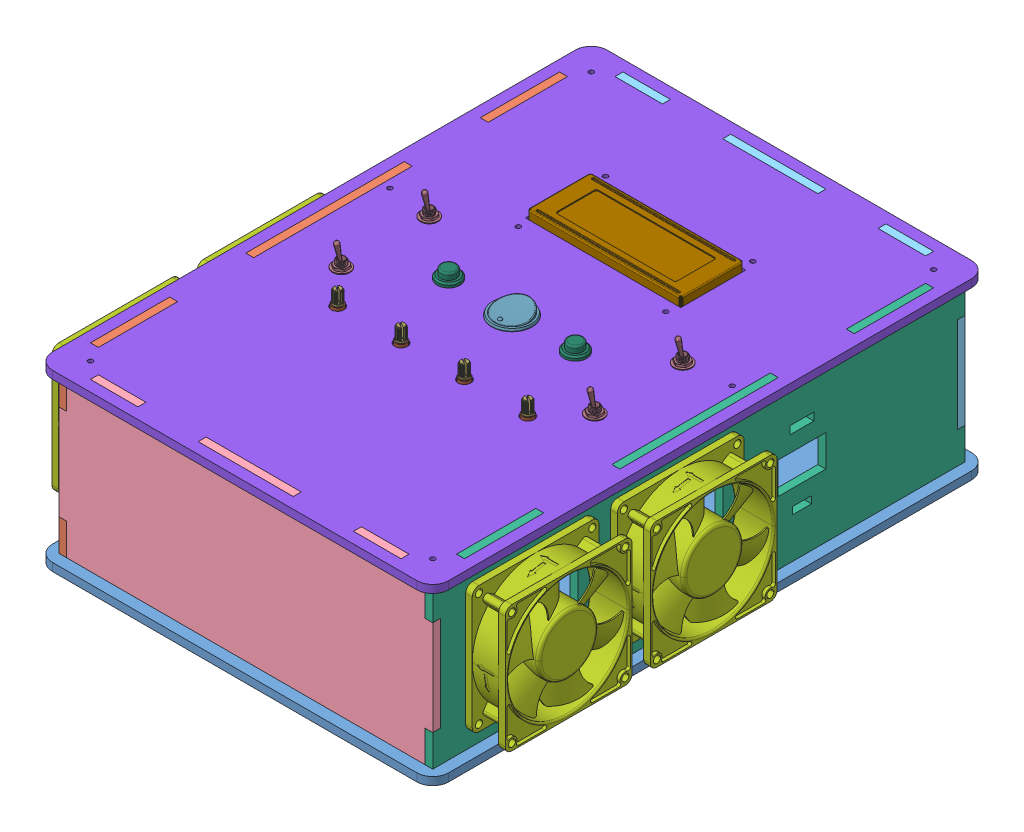
SolidWorks assembly Assem2, configuration Default. Lengths in mm.
Overall size (286.01 126.03 350).
54 component instances, 15 part files, 74 mates.
Components (placement in the parent):
- Bottom2-1: Bottom2 [Default] at (-2.3882 167.7912 456.2901) size (250 5 350)
- LargeEdge-1: LargeEdge [Default] at (9.6118 222.7912 281.2901) x (0 0 1) z (-1 0 0) size (336 110 5)
- PCB_Standoff-1: PCB_Standoff [Default] at (202.4618 172.7912 346.2901) size (4.59 40 5.3)
- PCB_Standoff-2: PCB_Standoff [Default] at (132.6118 172.7912 346.2901) size (4.59 40 5.3)
- PCB_Standoff-3: PCB_Standoff [Default] at (42.7618 172.7912 346.2901) size (4.59 40 5.3)
- PCB_Standoff-4: PCB_Standoff [Default] at (112.6118 172.7912 346.2901) size (4.59 40 5.3)
- PCB_Standoff-5: PCB_Standoff [Default] at (202.4618 172.7912 276.3101) size (4.59 40 5.3)
- PCB_Standoff-6: PCB_Standoff [Default] at (132.6118 172.7912 276.3101) size (4.59 40 5.3)
- PCB_Standoff-7: PCB_Standoff [Default] at (112.6118 172.7912 276.3101) size (4.59 40 5.3)
- PCB_Standoff-8: PCB_Standoff [Default] at (66.7318 172.7912 146.2901) size (4.59 40 5.3)
- PCB_Standoff-9: PCB_Standoff [Default] at (66.7318 172.7912 242.8101) size (4.59 40 5.3)
- PCB_Standoff-10: PCB_Standoff [Default] at (178.4918 172.7912 242.8101) size (4.59 40 5.3)
- PCB_Standoff-11: PCB_Standoff [Default] at (178.4918 172.7912 146.2901) size (4.59 40 5.3)
- PCB_Standoff-12: PCB_Standoff [Default] at (42.7618 172.7912 276.3101) size (4.59 40 5.3)
- SmallEdge-1: SmallEdge [Default] at (122.6118 222.7912 449.2901) x (0 0 -1) z (1 0 0) size (5 110 236)
- SmallEdge_OUTPUT-1: SmallEdge_OUTPUT [Default] at (122.6118 222.7912 118.2901) x (0 0 -1) z (1 0 0) size (5 110 236)
- LargeEdge_Right-1: LargeEdge_Right [Default] at (240.6118 222.7912 281.2901) x (0 0 1) z (-1 0 0) size (336 110 5)
- KARE AKS0YEL FAN_80x80x25 FAN.step-3: KARE AKS0YEL FAN_80x80x25 FAN.step [Default] at (253.1118 222.7912 388.5401) x (0 0 1) z (-1 0 0) size (80.72 80 25.01)
- KARE AKS0YEL FAN_80x80x25 FAN.step-4: KARE AKS0YEL FAN_80x80x25 FAN.step [Default] at (253.1118 222.7912 297.0401) x (0 0 1) z (-1 0 0) size (80.72 80 25.01)
- Top-1: Top [Default] at (-2.3882 272.7912 456.2901) size (250 5 350)
- LCD Display 2004.stp-1: LCD Display 2004.stp [Default] at (122.5938 271.1783 203.0951) size (98.07 13.66 59.94)
- PCB_Standoff_50mm-1: PCB_Standoff_50mm [Default] at (14.6118 172.7912 123.2901) x (0.790641 0 0.61228) z (-0.61228 0 0.790641) size (5.3 50 5.17)
- PCB_Standoff_50mm-2: PCB_Standoff_50mm [Default] at (14.6118 222.7912 123.2901) x (0.790641 0 0.61228) z (-0.61228 0 0.790641) size (5.3 50 5.17)
- PCB_Standoff_50mm-3: PCB_Standoff_50mm [Default] at (230.6118 222.7912 123.2901) size (5.3 50 5.17)
- PCB_Standoff_50mm-4: PCB_Standoff_50mm [Default] at (14.6118 222.7912 250.2901) size (5.3 50 5.17)
- PCB_Standoff_50mm-5: PCB_Standoff_50mm [Default] at (230.6118 172.7912 439.2901) size (5.3 50 5.17)
- PCB_Standoff_50mm-6: PCB_Standoff_50mm [Default] at (230.6118 222.7912 250.2901) size (5.3 50 5.17)
- PCB_Standoff_50mm-7: PCB_Standoff_50mm [Default] at (230.6118 172.7912 250.2901) size (5.3 50 5.17)
- PCB_Standoff_50mm-8: PCB_Standoff_50mm [Default] at (14.6118 172.7912 439.2901) size (5.3 50 5.17)
- PCB_Standoff_50mm-9: PCB_Standoff_50mm [Default] at (14.6118 172.7912 250.2901) size (5.3 50 5.17)
- PCB_Standoff_50mm-10: PCB_Standoff_50mm [Default] at (230.6118 172.7912 123.2901) size (5.3 50 5.17)
- PCB_Standoff_50mm-11: PCB_Standoff_50mm [Default] at (230.6118 222.7912 439.2901) size (5.3 50 5.17)
- PCB_Standoff_50mm-12: PCB_Standoff_50mm [Default] at (14.6118 222.7912 439.2901) size (5.3 50 5.17)
- KARE AKS0YEL FAN_80x80x25 FAN.step-5: KARE AKS0YEL FAN_80x80x25 FAN.step [Default] at (-7.8882 222.7912 297.0401) x (0 0 1) z (-1 0 0) size (80.72 80 25.01)
- KARE AKS0YEL FAN_80x80x25 FAN.step-6: KARE AKS0YEL FAN_80x80x25 FAN.step [Default] at (-7.8882 222.7912 388.5401) x (0 0 1) z (-1 0 0) size (80.72 80 25.01)
- WH148 PH1 Single-Joint Potentiometer.step-1: WH148 PH1 Single-Joint Potentiometer.step [Default] at (62.6118 270.7912 331.2901) x (0.999555 0 0.029816) z (0 1 0) size (16.9 26.15 23.9)
  - Base.step-1: Base.step [Default] at origin size (16.9 26.15 15.6)
  - Knob.step-1: Knob.step [Default] x (0.866025 0.5 0) z (0 0 1) size (5.8 5.8 8.2)
- WH148 PH1 Single-Joint Potentiometer.step-2: WH148 PH1 Single-Joint Potentiometer.step [Default] at (102.6118 270.7912 331.2901) x (1 0 0) z (0 1 0) size (16.9 26.15 23.9)
  - Base.step-1: Base.step [Default] at origin size (16.9 26.15 15.6)
  - Knob.step-1: Knob.step [Default] x (0.866025 0.5 0) z (0 0 1) size (5.8 5.8 8.2)
- WH148 PH1 Single-Joint Potentiometer.step-3: WH148 PH1 Single-Joint Potentiometer.step [Default] at (142.6118 270.7912 331.2901) x (1 0 0) z (0 1 0) size (16.9 26.15 23.9)
  - Base.step-1: Base.step [Default] at origin size (16.9 26.15 15.6)
  - Knob.step-1: Knob.step [Default] x (0.866025 0.5 0) z (0 0 1) size (5.8 5.8 8.2)
- WH148 PH1 Single-Joint Potentiometer.step-4: WH148 PH1 Single-Joint Potentiometer.step [Default] at (182.6118 270.7912 331.2901) x (1 0 0) z (0 1 0) size (16.9 26.15 23.9)
  - Base.step-1: Base.step [Default] at origin size (16.9 26.15 15.6)
  - Knob.step-1: Knob.step [Default] x (0.866025 0.5 0) z (0 0 1) size (5.8 5.8 8.2)
- MTS-102.step-6: MTS-102.step [Default] at (42.6118 273.7912 253.5562) x (0 0 -1) z (1 0 0) size (13.2 33.53 12)
- MTS-102.step-7: MTS-102.step [Default] at (42.6118 273.7912 309.024) x (0 0 -1) z (1 0 0) size (13.2 33.53 12)
- MTS-102.step-8: MTS-102.step [Default] at (202.6118 273.7912 253.5562) x (0 0 -1) z (1 0 0) size (13.2 33.53 12)
- MTS-102.step-9: MTS-102.step [Default] at (202.6118 273.7912 309.024) x (0 0 -1) z (1 0 0) size (13.2 33.53 12)
- rocker switch.step-4: rocker switch.step [Default] at (122.6118 277.7912 281.2901) x (0.999998 0 -0.002169) z (-0.002169 0 -0.999998) size (25.4 25.47 25.4)
- Push Button.step-3: Push Button.step [Default] at (82.6118 268.6912 281.2901) x (1 0 0) z (0 1 0) size (16.28 16.39 30.3)
- Push Button.step-4: Push Button.step [Default] at (162.6118 268.6912 281.2901) x (1 0 0) z (0 1 0) size (16.28 16.39 30.3)
Mates (geometry in assembly coordinates):
- Coincident10: coincident anti-aligned: circle of Bottom2-1; circle of PCB_Standoff-1
- Coincident11: coincident anti-aligned: circle of Bottom2-1; circle of PCB_Standoff-2
- Coincident12: coincident aligned: circle of Bottom2-1; circle of PCB_Standoff-3
- Coincident13: coincident aligned: circle of Bottom2-1; circle of PCB_Standoff-4
- Coincident14: coincident anti-aligned: circle of Bottom2-1; circle of PCB_Standoff-5
- Coincident15: coincident anti-aligned: circle of Bottom2-1; circle of PCB_Standoff-6
- Coincident16: coincident aligned: circle of Bottom2-1; circle of PCB_Standoff-12
- Coincident18: coincident aligned: circle of Bottom2-1; circle of PCB_Standoff-10
- Coincident19: coincident aligned: circle of Bottom2-1; circle of PCB_Standoff-9
- Coincident20: coincident aligned: circle of Bottom2-1; circle of PCB_Standoff-11
- Coincident21: coincident aligned: circle of Bottom2-1; circle of PCB_Standoff-8
- Coincident25: coincident aligned: circle of Bottom2-1; circle of PCB_Standoff-7
- Coincident28: coincident anti-aligned: plane of Bottom2-1 through (220.6118 172.7912 456.2901) normal (-1 0 0); plane of SmallEdge_OUTPUT-1 through (220.6118 222.7912 113.2901) normal (1 0 0)
- Coincident29: coincident anti-aligned: plane of Bottom2-1 through (-2.3882 172.7912 456.2901) normal (0 1 0); plane of SmallEdge_OUTPUT-1 through (122.6118 172.7912 113.2901) normal (0 -1 0)
- Coincident30: coincident anti-aligned: plane of Bottom2-1 through (-2.3882 172.7912 118.2901) normal (0 0 -1); plane of SmallEdge_OUTPUT-1 through (122.6118 222.7912 118.2901) normal (0 0 1)
- Coincident31: coincident anti-aligned: plane of Bottom2-1 through (-2.3882 172.7912 379.2901) normal (0 0 1); plane of LargeEdge-1 through (4.6118 222.7912 379.2901) normal (0 0 -1)
- Coincident32: coincident anti-aligned: plane of Bottom2-1 through (9.6118 172.7912 456.2901) normal (-1 0 0); plane of LargeEdge-1 through (9.6118 222.7912 281.2901) normal (1 0 0)
- Coincident33: coincident anti-aligned: plane of Bottom2-1 through (-2.3882 172.7912 456.2901) normal (0 1 0); plane of LargeEdge-1 through (4.6118 172.7912 281.2901) normal (0 -1 0)
- Coincident34: coincident anti-aligned: plane of Bottom2-1 through (24.6118 172.7912 456.2901) normal (1 0 0); plane of SmallEdge-1 through (24.6118 172.7912 444.2901) normal (-1 0 0)
- Coincident35: coincident anti-aligned: plane of Bottom2-1 through (-2.3882 172.7912 444.2901) normal (0 0 1); plane of SmallEdge-1 through (122.6118 222.7912 444.2901) normal (0 0 -1)
- Coincident36: coincident anti-aligned: plane of Bottom2-1 through (-2.3882 172.7912 456.2901) normal (0 1 0); plane of SmallEdge-1 through (122.6118 172.7912 444.2901) normal (0 -1 0)
- Coincident37: coincident anti-aligned: plane of Bottom2-1 through (-2.3882 172.7912 429.2901) normal (0 0 -1); plane of LargeEdge_Right-1 through (235.6118 222.7912 429.2901) normal (0 0 1)
- Coincident38: coincident anti-aligned: plane of Bottom2-1 through (235.6118 172.7912 456.2901) normal (1 0 0); plane of LargeEdge_Right-1 through (235.6118 222.7912 281.2901) normal (-1 0 0)
- Coincident39: coincident anti-aligned: plane of Bottom2-1 through (-2.3882 172.7912 456.2901) normal (0 1 0); plane of LargeEdge_Right-1 through (235.6118 172.7912 281.2901) normal (0 -1 0)
- Concentric11: concentric aligned: circle of LargeEdge_Right-1; circle of KARE AKS0YEL FAN_80x80x25 FAN.step-3
- Concentric12: concentric aligned: circle of LargeEdge_Right-1; circle of KARE AKS0YEL FAN_80x80x25 FAN.step-3
- Coincident42: coincident anti-aligned: plane of LargeEdge_Right-1 through (240.6118 222.7912 281.2901) normal (1 0 0); plane of KARE AKS0YEL FAN_80x80x25 FAN.step-3 through (240.6118 222.7912 388.5401) normal (-1 0 0)
- Concentric13: concentric aligned: circle of LargeEdge_Right-1; circle of KARE AKS0YEL FAN_80x80x25 FAN.step-4
- Concentric14: concentric aligned: circle of LargeEdge_Right-1; circle of KARE AKS0YEL FAN_80x80x25 FAN.step-4
- Coincident43: coincident anti-aligned: plane of LargeEdge_Right-1 through (240.6118 222.7912 281.2901) normal (1 0 0); plane of KARE AKS0YEL FAN_80x80x25 FAN.step-4 through (240.6118 222.7912 297.0401) normal (-1 0 0)
- Coincident59: coincident anti-aligned: plane of LargeEdge_Right-1 through (235.6118 272.7912 281.2901) normal (0 1 0); plane of Top-1 through (-2.3882 272.7912 447.8511) normal (0 -1 0)
- Concentric25: concentric anti-aligned: cylinder of Top-1 through (76.1118 277.7912 167.3511) axis (0 -1 0) radius 1.5; cylinder of LCD Display 2004.stp-1 through (76.1118 271.1783 167.3511) axis (0 1 0) radius 1.6764
- Parallel7: parallel anti-aligned: plane of Top-1 through (171.6118 277.7912 447.8511) normal (-1 0 0); plane of LCD Display 2004.stp-1 through (170.9681 281.7828 213.3886) normal (1 0 0)
- Coincident61: coincident anti-aligned: plane of Top-1 through (-2.3882 272.7912 447.8511) normal (0 -1 0); plane of LCD Display 2004.stp-1 through (122.5938 272.7912 194.6561) normal (0 1 0)
- Coincident64: coincident aligned: circle of Bottom2-1; circle of PCB_Standoff_50mm-1
- Coincident65: coincident aligned: circle of PCB_Standoff_50mm-1; circle of PCB_Standoff_50mm-2
- Coincident66: coincident aligned: circle of Bottom2-1; circle of PCB_Standoff_50mm-9
- Coincident67: coincident aligned: circle of PCB_Standoff_50mm-4; circle of PCB_Standoff_50mm-9
- Coincident68: coincident anti-aligned: circle of Bottom2-1; circle of PCB_Standoff_50mm-8
- Coincident69: coincident aligned: circle of Bottom2-1; circle of PCB_Standoff_50mm-5
- Coincident70: coincident anti-aligned: circle of Bottom2-1; circle of PCB_Standoff_50mm-7
- Coincident71: coincident anti-aligned: circle of Bottom2-1; circle of PCB_Standoff_50mm-10
- Coincident72: coincident aligned: circle of PCB_Standoff_50mm-3; circle of PCB_Standoff_50mm-10
- Coincident73: coincident aligned: circle of PCB_Standoff_50mm-6; circle of PCB_Standoff_50mm-7
- Coincident74: coincident aligned: circle of PCB_Standoff_50mm-5; circle of PCB_Standoff_50mm-11
- Coincident75: coincident aligned: circle of PCB_Standoff_50mm-8; circle of PCB_Standoff_50mm-12
- Concentric26: concentric anti-aligned: circle of LargeEdge-1; circle of KARE AKS0YEL FAN_80x80x25 FAN.step-5
- Concentric28: concentric anti-aligned: circle of LargeEdge-1; circle of KARE AKS0YEL FAN_80x80x25 FAN.step-5
- Coincident80: coincident anti-aligned: plane of LargeEdge-1 through (4.6118 222.7912 281.2901) normal (-1 0 0); plane of KARE AKS0YEL FAN_80x80x25 FAN.step-5 through (4.6118 222.7912 297.0401) normal (1 0 0)
- Concentric29: concentric anti-aligned: circle of LargeEdge-1; circle of KARE AKS0YEL FAN_80x80x25 FAN.step-6
- Concentric30: concentric anti-aligned: circle of LargeEdge-1; circle of KARE AKS0YEL FAN_80x80x25 FAN.step-6
- Coincident81: coincident anti-aligned: plane of LargeEdge-1 through (4.6118 222.7912 281.2901) normal (-1 0 0); plane of KARE AKS0YEL FAN_80x80x25 FAN.step-6 through (4.6118 222.7912 388.5401) normal (1 0 0)
- Concentric32: concentric anti-aligned: circle of Top-1; circle of WH148 PH1 Single-Joint Potentiometer.step-1/Base.step-1
- Concentric33: concentric anti-aligned: circle of Top-1; circle of WH148 PH1 Single-Joint Potentiometer.step-2/Base.step-1
- Coincident82: coincident anti-aligned: plane of Top-1 through (-2.3882 272.7912 447.8511) normal (0 -1 0); plane of WH148 PH1 Single-Joint Potentiometer.step-2/Base.step-1 through (102.6118 272.7912 322.8511) normal (0 1 0)
- Coincident83: coincident anti-aligned: plane of Top-1 through (-2.3882 272.7912 447.8511) normal (0 -1 0); plane of WH148 PH1 Single-Joint Potentiometer.step-1/Base.step-1 through (62.6118 272.7912 322.8511) normal (0 1 0)
- Concentric34: concentric aligned: circle of Top-1; circle of WH148 PH1 Single-Joint Potentiometer.step-3/Base.step-1
- Coincident84: coincident anti-aligned: plane of Top-1 through (-2.3882 272.7912 447.8511) normal (0 -1 0); plane of WH148 PH1 Single-Joint Potentiometer.step-3/Base.step-1 through (142.6118 272.7912 322.8511) normal (0 1 0)
- Concentric35: concentric aligned: circle of Top-1; circle of WH148 PH1 Single-Joint Potentiometer.step-4/Base.step-1
- Coincident85: coincident anti-aligned: plane of Top-1 through (-2.3882 272.7912 447.8511) normal (0 -1 0); plane of WH148 PH1 Single-Joint Potentiometer.step-4/Base.step-1 through (182.6118 272.7912 322.8511) normal (0 1 0)
- Coincident86: coincident anti-aligned: plane of Top-1 through (-2.3882 277.7912 447.8511) normal (0 1 0); plane of MTS-102.step-6 through (42.6118 277.7912 245.1172) normal (0 -1 0)
- Concentric36: concentric anti-aligned: circle of Top-1; circle of MTS-102.step-6
- Coincident87: coincident anti-aligned: plane of Top-1 through (-2.3882 277.7912 447.8511) normal (0 1 0); plane of MTS-102.step-7 through (42.6118 277.7912 300.585) normal (0 -1 0)
- Concentric37: concentric aligned: circle of Top-1; circle of MTS-102.step-7
- Coincident88: coincident anti-aligned: plane of Top-1 through (-2.3882 277.7912 447.8511) normal (0 1 0); plane of MTS-102.step-8 through (202.6118 277.7912 245.1172) normal (0 -1 0)
- Concentric38: concentric aligned: circle of Top-1; circle of MTS-102.step-8
- Coincident89: coincident anti-aligned: plane of Top-1 through (-2.3882 277.7912 447.8511) normal (0 1 0); plane of MTS-102.step-9 through (202.6118 277.7912 300.585) normal (0 -1 0)
- Concentric39: concentric anti-aligned: circle of Top-1; circle of MTS-102.step-9
- Concentric40: concentric anti-aligned: circle of Top-1; circle of rocker switch.step-4
- Coincident90: coincident anti-aligned: plane of Top-1 through (-2.3882 277.7912 447.8511) normal (0 1 0); plane of rocker switch.step-4 through (122.6118 277.7912 272.8511) normal (0 -1 0)
- Coincident91: coincident anti-aligned: circle of Top-1; circle of Push Button.step-4
- Coincident92: coincident aligned: circle of Top-1; circle of Push Button.step-3
- Coincident93: coincident anti-aligned: plane of LargeEdge-1 through (9.6118 222.7912 281.2901) normal (1 0 0); plane of Top-1 through (9.6118 277.7912 456.2901) normal (-1 0 0)
- Coincident94: coincident anti-aligned: plane of LargeEdge-1 through (4.6118 222.7912 133.2901) normal (0 0 -1); plane of Top-1 through (-2.3882 277.7912 133.2901) normal (0 0 1)
